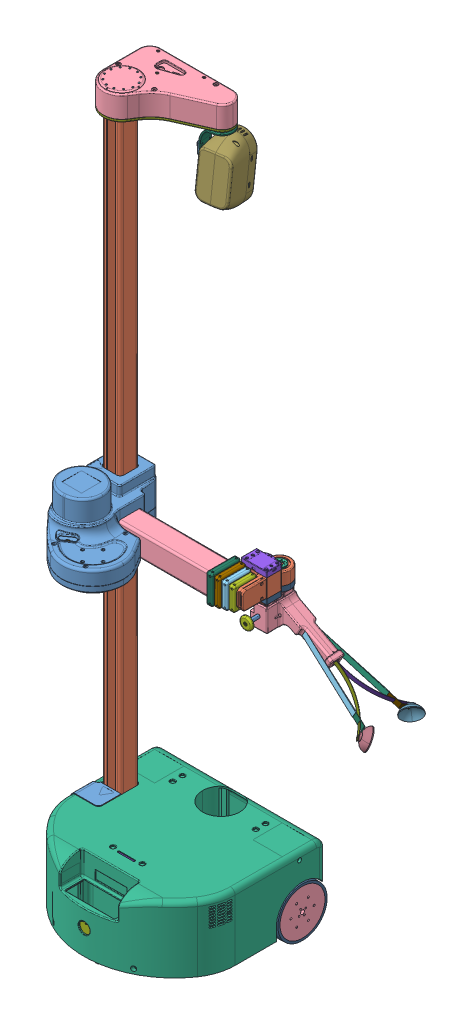
SolidWorks assembly ASM-stretch_re2_nina, configuration Default. Lengths in mm.
Overall size (574.57 1429.23 345.9).
120 component instances, 97 part files, 14 mates.
Components (placement in the parent):
- ASM-base_module.step-1: ASM-base_module.step [Default] at (9.1565 -1330.6492 124.8432) x (1 0 0) z (0 1 0) size (352.17 345.9 1378.51)
  - ASM-base_module1.STEP-1: ASM-base_module1.STEP [Default] at origin size (2.05 13.46 21.35)
  - ASM-base_module2.STEP-1: ASM-base_module2.STEP [Default] at origin size (0.01 36.41 25.92)
  - ASM-base_module3.STEP-1: ASM-base_module3.STEP [Default] at origin size (6.01 6.54 4.61)
  - ASM-base_module4.STEP-1: ASM-base_module4.STEP [Default] at origin size (25.56 91.93 91.93)
  - ASM-base_module5.STEP-1: ASM-base_module5.STEP [Default] at origin size (6 3.9 3.75)
  - ASM-base_module6.STEP-1: ASM-base_module6.STEP [Default] at origin size (352.17 325 150.78)
  - ASM-base_module7.STEP-1: ASM-base_module7.STEP [Default] at origin size (13.8 55.1 43.54)
  - ASM-base_module8.STEP-1: ASM-base_module8.STEP [Default] at origin size (6 3.75 3.9)
  - ASM-base_module9.STEP-1: ASM-base_module9.STEP [Default] at origin size (25.41 123.2 123.2)
  - ASM-base_module10.STEP-1: ASM-base_module10.STEP [Default] at origin size (22.01 60.76 15.75)
  - ASM-base_module11.STEP-1: ASM-base_module11.STEP [Default] at origin size (0.01 35.01 28.06)
  - ASM-base_module12.STEP-1: ASM-base_module12.STEP [Default] at origin size (8.4 7.44 8.82)
  - ASM-base_module13.STEP-1: ASM-base_module13.STEP [Default] at origin size (0.01 35.22 1.01)
  - ASM-base_module14.STEP-1: ASM-base_module14.STEP [Default] at origin size (0.01 20.82 20.37)
  - ASM-base_module15.STEP-1: ASM-base_module15.STEP [Default] at origin size (8.4 6.85 11.7)
  - ASM-base_module16.STEP-1: ASM-base_module16.STEP [Default] at origin size (332.01 319.06 14.35)
  - ASM-base_module17.STEP-1: ASM-base_module17.STEP [Default] at origin size (8.4 7.35 9.57)
  - ASM-base_module18.STEP-1: ASM-base_module18.STEP [Default] at origin size (22.01 60.76 15.75)
  - ASM-base_module19.STEP-1: ASM-base_module19.STEP [Default] at origin size (57.07 47.59 136.87)
  - ASM-base_module20.STEP-1: ASM-base_module20.STEP [Default] at origin size (38.14 38.14 1268.02)
  - ASM-base_module21.STEP-1: ASM-base_module21.STEP [Default] at origin size (25.56 102.18 102.18)
  - ASM-base_module22.STEP-1: ASM-base_module22.STEP [Default] at origin size (27.89 20.39 20.39)
  - ASM-base_module23.STEP-1: ASM-base_module23.STEP [Default] at origin size (8.4 7.6 9.1)
  - ASM-base_module24.STEP-1: ASM-base_module24.STEP [Default] at origin size (6 3.75 3.53)
  - ASM-base_module25.STEP-1: ASM-base_module25.STEP [Default] at origin size (0.01 17.39 23.47)
  - ASM-base_module26.STEP-1: ASM-base_module26.STEP [Default] at origin size (21.07 103.14 103.14)
  - ASM-base_module27.STEP-1: ASM-base_module27.STEP [Default] at origin size (8.4 5.66 7.84)
  - ASM-base_module28.STEP-1: ASM-base_module28.STEP [Default] at origin size (25.41 138.8 138.8)
  - ASM-base_module29.STEP-1: ASM-base_module29.STEP [Default] at origin size (19.01 2.01 2.01)
  - ASM-base_module30.STEP-1: ASM-base_module30.STEP [Default] at origin size (0.01 3.01 115.61)
  - ASM-base_module31.STEP-1: ASM-base_module31.STEP [Default] at origin size (25.49 120.63 120.63)
  - ASM-base_module32.STEP-1: ASM-base_module32.STEP [Default] at origin size (13.8 52.4 43.41)
  - ASM-base_module33.STEP-1: ASM-base_module33.STEP [Default] at origin size (8.4 9.77 9.42)
  - ASM-base_module34.STEP-1: ASM-base_module34.STEP [Default] at origin size (29.85 49.98 45.18)
  - ASM-base_module35.STEP-1: ASM-base_module35.STEP [Default] at origin size (38.71 7.71 0.01)
  - ASM-base_module36.STEP-1: ASM-base_module36.STEP [Default] at origin size (7.64 2.75 7.13)
  - ASM-base_module37.STEP-1: ASM-base_module37.STEP [Default] at origin size (0.01 17.39 23.47)
  - ASM-base_module38.STEP-1: ASM-base_module38.STEP [Default] at origin size (0.01 91.94 91.94)
  - ASM-base_module39.STEP-1: ASM-base_module39.STEP [Default] at origin size (6 3.9 3.75)
- ASM-head_module.STEP-1: ASM-head_module.STEP [Default] at (-30.1698 -72.0673 12.5567) size (192.75 55.42 133.8)
  - SIM-630_head_shell_light_pipes.STEP-1: SIM-630_head_shell_light_pipes.STEP [Default] at (-125.0983 70.6549 49.8978) size (192.75 46.56 133.8)
    - BIG-924_head_shell.STEP-1: BIG-924_head_shell.STEP [Default] at (0 49.7625 0) x (1 0 0) z (0 1 0) size (192.75 133.8 45.8)
    - HDW-923_LightPipe_LFB025CTP.STEP-1: HDW-923_LightPipe_LFB025CTP.STEP [Default] at (-22.9378 51.8 9.4195) x (0 1 0) z (-0.203299 0 0.979117) size (7.11 3.3 3.3)
    - HDW-923_LightPipe_LFB025CTP.STEP-2: HDW-923_LightPipe_LFB025CTP.STEP [Default] at (-6.5158 51.8 -25.8667) x (0 1 0) z (0.471956 0 0.881622) size (7.11 3.3 3.3)
    - HDW-923_LightPipe_LFB025CTP.STEP-3: HDW-923_LightPipe_LFB025CTP.STEP [Default] at (7.7778 51.8 -27.1304) x (0 1 0) z (-0.504358 0 -0.863495) size (7.11 3.3 3.3)
    - HDW-923_LightPipe_LFB025CTP.STEP-4: HDW-923_LightPipe_LFB025CTP.STEP [Default] at (-14.7362 51.8 21.1114) x (0 1 0) z (-0.970654 0 0.24048) size (7.11 3.3 3.3)
    - HDW-923_LightPipe_LFB025CTP.STEP-5: HDW-923_LightPipe_LFB025CTP.STEP [Default] at (-24.1362 51.8 -4.7944) x (0 1 0) z (0.380757 0 0.924675) size (7.11 3.3 3.3)
    - HDW-923_LightPipe_LFB025CTP.STEP-6: HDW-923_LightPipe_LFB025CTP.STEP [Default] at (-18.133 51.8 -17.7146) x (0 1 0) z (0.667843 0 0.744302) size (7.11 3.3 3.3)
    - HDW-923_LightPipe_LFB025CTP.STEP-7: HDW-923_LightPipe_LFB025CTP.STEP [Default] at (28.9074 51.8 -9.4109) x (0 1 0) z (-0.414071 0 0.910245) size (7.11 3.3 3.3)
    - HDW-923_LightPipe_LFB025CTP.STEP-8: HDW-923_LightPipe_LFB025CTP.STEP [Default] at (30.1657 51.8 4.8066) x (0 1 0) z (-0.782358 0 -0.622829) size (7.11 3.3 3.3)
    - HDW-923_LightPipe_LFB025CTP.STEP-9: HDW-923_LightPipe_LFB025CTP.STEP [Default] at (20.693 51.8 -21.1114) x (0 1 0) z (-0.514508 0 -0.857486) size (7.11 3.3 3.3)
    - HDW-923_LightPipe_LFB025CTP.STEP-10: HDW-923_LightPipe_LFB025CTP.STEP [Default] at (24.0898 51.8 17.7146) x (0 1 0) z (-0.414071 0 0.910245) size (7.11 3.3 3.3)
    - HDW-923_LightPipe_LFB025CTP.STEP-11: HDW-923_LightPipe_LFB025CTP.STEP [Default] at (-1.8022 51.8 27.1343) x (0 1 0) z (0.974021 0 0.226458) size (7.11 3.3 3.3)
    - HDW-923_LightPipe_LFB025CTP.STEP-12: HDW-923_LightPipe_LFB025CTP.STEP [Default] at (12.3407 51.8 25.8882) x (0 1 0) z (-0.414071 0 0.910245) size (7.11 3.3 3.3)
    - HDW-A01_5288T111_Oil-Resistant Buna-N Backup Rings_5288T111.STEP-1: HDW-A01_5288T111_Oil-Resistant Buna-N Backup Rings_5288T111.STEP [Default] at (5.1887 44.2723 32.1986) x (-0.310775 0 0.950484) z (0.950484 0 0.310775) size (5.92 1.24 5.92)
    - HDW-A01_5288T111_Oil-Resistant Buna-N Backup Rings_5288T111.STEP-2: HDW-A01_5288T111_Oil-Resistant Buna-N Backup Rings_5288T111.STEP [Default] at (0.8407 44.2723 -32.2627) x (-0.971613 0 0.236575) z (0.236575 0 0.971613) size (5.92 1.24 5.92)
    - HDW-A01_5288T111_Oil-Resistant Buna-N Backup Rings_5288T111.STEP-3: HDW-A01_5288T111_Oil-Resistant Buna-N Backup Rings_5288T111.STEP [Default] at (-29.2159 44.2723 2.142) x (-0.310775 0 0.950484) z (0.950484 0 0.310775) size (5.92 1.24 5.92)
    - HDW-A01_5288T111_Oil-Resistant Buna-N Backup Rings_5288T111.STEP-4: HDW-A01_5288T111_Oil-Resistant Buna-N Backup Rings_5288T111.STEP [Default] at (35.2453 44.2723 -2.2061) x (0.971309 0 0.237823) z (0.237823 0 -0.971309) size (5.92 1.24 5.92)
  - BIG-926_head_bottom_plate_simple.STEP-1: BIG-926_head_bottom_plate_simple.STEP [Default] at (-125.0983 70.6549 49.8978) x (0 0 1) z (0 -1 0) size (133.8 192.72 8.51)
  - HDW-920_head_pan_shaft.STEP-1: HDW-920_head_pan_shaft.STEP [Default] at (9.9017 111.1758 -23.2022) x (0 1 0) z (0.414693 0 0.909961) size (40.5 24.99 24.99)
  - VND-821_head_mount_plate.STEP-1: VND-821_head_mount_plate.STEP [Default] at (-125.0983 70.9908 49.8978) x (0 0 -1) z (0 1 0) size (73.84 73.84 3)
- ASM_head_tilt_hanger.step-1: ASM_head_tilt_hanger.step [Default] at (-5.771 -6.9174 -10.9643) x (0.988973 0 -0.148096) z (0.148096 0 0.988973) size (62.97 69.82 45.01)
  - ASM_head_tilt_hanger1.STEP-1: ASM_head_tilt_hanger1.STEP [Default] at origin size (0.01 1.84 1.84)
  - ASM_head_tilt_hanger2.STEP-1: ASM_head_tilt_hanger2.STEP [Default] at origin size (0.01 1.84 1.84)
  - ASM_head_tilt_hanger3.STEP-1: ASM_head_tilt_hanger3.STEP [Default] at origin size (0.01 1.84 1.84)
  - ASM_head_tilt_hanger4.STEP-1: ASM_head_tilt_hanger4.STEP [Default] at origin size (7.22 2.09 7.22)
  - ASM_head_tilt_hanger5.STEP-1: ASM_head_tilt_hanger5.STEP [Default] at origin size (11.4 31.82 26.47)
  - ASM_head_tilt_hanger6.STEP-1: ASM_head_tilt_hanger6.STEP [Default] at origin size (55.12 69.82 45.01)
  - ASM_head_tilt_hanger7.STEP-1: ASM_head_tilt_hanger7.STEP [Default] at origin size (2.97 6.64 6.64)
  - ASM_head_tilt_hanger8.STEP-1: ASM_head_tilt_hanger8.STEP [Default] at origin size (2.97 6.64 6.64)
  - ASM_head_tilt_hanger9.STEP-1: ASM_head_tilt_hanger9.STEP [Default] at origin size (2.97 6.64 6.64)
- SUB-202_head_tilt_simple.step-1: SUB-202_head_tilt_simple.step [Default] at (-21.5187 -75.739 -52.7585) x (-0.988973 0 0.148096) z (-0.14655 -0.144108 -0.97865) size (65.06 133.38 73.8)
  - SUB-202_head_tilt_simple1.STEP-1: SUB-202_head_tilt_simple1.STEP [Default] at origin size (7.15 7.51 7.51)
  - SUB-202_head_tilt_simple2.STEP-1: SUB-202_head_tilt_simple2.STEP [Default] at origin size (16 81 0.56)
  - SUB-202_head_tilt_simple3.STEP-1: SUB-202_head_tilt_simple3.STEP [Default] at origin size (32.75 27 27)
  - SUB-202_head_tilt_simple4.STEP-1: SUB-202_head_tilt_simple4.STEP [Default] at origin size (3.8 7.01 3.01)
  - SUB-202_head_tilt_simple5.STEP-1: SUB-202_head_tilt_simple5.STEP [Default] at origin size (3.8 7.01 3.01)
  - SUB-202_head_tilt_simple6.STEP-1: SUB-202_head_tilt_simple6.STEP [Default] at origin size (48.91 33.18 33.18)
  - SUB-202_head_tilt_simple7.STEP-1: SUB-202_head_tilt_simple7.STEP [Default] at origin size (3.8 7.01 3.01)
  - SUB-202_head_tilt_simple8.STEP-1: SUB-202_head_tilt_simple8.STEP [Default] at origin size (9.01 6.36 3.19)
  - SUB-202_head_tilt_simple9.STEP-1: SUB-202_head_tilt_simple9.STEP [Default] at origin size (3.8 7.01 3.01)
  - SUB-202_head_tilt_simple10.STEP-1: SUB-202_head_tilt_simple10.STEP [Default] at origin size (56.31 116.27 4.3)
  - SUB-202_head_tilt_simple11.STEP-1: SUB-202_head_tilt_simple11.STEP [Default] at origin size (23.01 2.51 0.01)
  - SUB-202_head_tilt_simple12.STEP-1: SUB-202_head_tilt_simple12.STEP [Default] at origin size (65.06 130.97 69.23)
  - SUB-202_head_tilt_simple13.STEP-1: SUB-202_head_tilt_simple13.STEP [Default] at origin size (39.68 92.75 30.1)
  - SUB-202_head_tilt_simple14.STEP-1: SUB-202_head_tilt_simple14.STEP [Default] at origin size (27.52 27.52 27.52)
- ASM_Arm_with_Wrist_simple.step-1: ASM_Arm_with_Wrist_simple.step [Default] at (-123.1677 -699.0905 99.7103) size (377.58 155.09 260.45)
  - ASM_Arm_with_Wrist_simple1.STEP-1: ASM_Arm_with_Wrist_simple1.STEP [Default] at origin size (13.01 59.49 59.46)
  - ASM_Arm_with_Wrist_simple2.STEP-1: ASM_Arm_with_Wrist_simple2.STEP [Default] at origin size (100.01 4.01 96.01)
  - ASM_Arm_with_Wrist_simple3.STEP-1: ASM_Arm_with_Wrist_simple3.STEP [Default] at origin size (0.01 34.01 34.01)
  - ASM_Arm_with_Wrist_simple4.STEP-1: ASM_Arm_with_Wrist_simple4.STEP [Default] at origin size (10.01 0.01 10.01)
  - ASM_Arm_with_Wrist_simple5.STEP-1: ASM_Arm_with_Wrist_simple5.STEP [Default] at origin size (191.75 155.09 244.07)
  - ASM_Arm_with_Wrist_simple6.STEP-1: ASM_Arm_with_Wrist_simple6.STEP [Default] at origin size (78.93 57.83 130.52)
  - ASM_Arm_with_Wrist_simple7.STEP-1: ASM_Arm_with_Wrist_simple7.STEP [Default] at origin size (177.19 121.67 235.79)
  - ASM_Arm_with_Wrist_simple8.STEP-1: ASM_Arm_with_Wrist_simple8.STEP [Default] at origin size (244.12 74.4 74.4)
  - ASM_Arm_with_Wrist_simple9.STEP-1: ASM_Arm_with_Wrist_simple9.STEP [Default] at origin size (13.01 51.36 51.36)
  - ASM_Arm_with_Wrist_simple10.STEP-1: ASM_Arm_with_Wrist_simple10.STEP [Default] at origin size (32.66 43.09 32.66)
  - ASM_Arm_with_Wrist_simple11.STEP-1: ASM_Arm_with_Wrist_simple11.STEP [Default] at origin size (13.01 47.36 47.36)
  - ASM_Arm_with_Wrist_simple12.STEP-1: ASM_Arm_with_Wrist_simple12.STEP [Default] at origin size (52.51 20.59 50.95)
  - ASM_Arm_with_Wrist_simple13.STEP-1: ASM_Arm_with_Wrist_simple13.STEP [Default] at origin size (13.01 55.26 55.26)
  - ASM_Arm_with_Wrist_simple14.STEP-1: ASM_Arm_with_Wrist_simple14.STEP [Default] at origin size (53.78 12.96 73.76)
- HDW-911_gripper_mount_bracket.STEP-1: HDW-911_gripper_mount_bracket.STEP [Default] at (123.1348 -627.1623 -27.3033) x (0 1 0) z (0.027951 0 0.999609) size (14 28 56.75)
  - VND-817_gripper_mount_bracket.STEP-1: VND-817_gripper_mount_bracket.STEP [Default] at (-122.2701 -0.2167 85.7868) size (11.5 28 56.75)
  - VND-818_MPP-1.5mm-4-PennEngineering.STEP-1: VND-818_MPP-1.5mm-4-PennEngineering.STEP [Default] at (-104.2701 -7.335 37.0133) size (4 2.24 2.24)
  - VND-818_MPP-1.5mm-4-PennEngineering.STEP-2: VND-818_MPP-1.5mm-4-PennEngineering.STEP [Default] at (-104.2701 -7.335 51.0603) size (4 2.24 2.24)
- ASM-207_Gripper_Simple.step-1: ASM-207_Gripper_Simple.step [Default] at (251.416 -808.1884 -3.9687) x (0.999609 0 -0.027951) z (0.027951 0 0.999609) size (261.51 171.11 139.86)
  - ASM-207_Gripper_Simple1.STEP-1: ASM-207_Gripper_Simple1.STEP [Default] at origin size (35.66 45.77 42.41)
  - ASM-207_Gripper_Simple2.STEP-1: ASM-207_Gripper_Simple2.STEP [Default] at origin size (38.03 42.61 42.49)
  - ASM-207_Gripper_Simple3.STEP-1: ASM-207_Gripper_Simple3.STEP [Default] at origin size (167.87 105.91 44.86)
  - ASM-207_Gripper_Simple4.STEP-1: ASM-207_Gripper_Simple4.STEP [Default] at origin size (111.68 70.98 65.43)
  - ASM-207_Gripper_Simple5.STEP-1: ASM-207_Gripper_Simple5.STEP [Default] at origin size (111.76 70.98 65.24)
  - ASM-207_Gripper_Simple6.STEP-1: ASM-207_Gripper_Simple6.STEP [Default] at origin size (168.93 105.91 49.34)
  - ASM-207_Gripper_Simple7.STEP-1: ASM-207_Gripper_Simple7.STEP [Default] at origin size (7.49 7.49 25.15)
  - ASM-207_Gripper_Simple8.STEP-1: ASM-207_Gripper_Simple8.STEP [Default] at origin size (0.65 0.01 4.01)
  - ASM-207_Gripper_Simple9.STEP-1: ASM-207_Gripper_Simple9.STEP [Default] at origin size (0.65 0.65 0.01)
  - ASM-207_Gripper_Simple10.STEP-1: ASM-207_Gripper_Simple10.STEP [Default] at origin size (141.61 96.71 65.91)
  - ASM-207_Gripper_Simple11.STEP-1: ASM-207_Gripper_Simple11.STEP [Default] at origin size (144.09 94.9 39.31)
  - ASM-207_Gripper_Simple12.STEP-1: ASM-207_Gripper_Simple12.STEP [Default] at origin size (144.09 94.9 38.54)
  - ASM-207_Gripper_Simple13.STEP-1: ASM-207_Gripper_Simple13.STEP [Default] at origin size (25.66 25.66 5.66)
Mates (geometry in assembly coordinates):
- Concentric4: concentric: cylinder of ASM-base_module.step-1/ASM-base_module20.STEP-1 through (-169.2181 -1266.0765 47.2919) axis (0 1 0) radius 2.1; cylinder of ASM-head_module.STEP-1/VND-821_head_mount_plate.STEP-1 through (-169.2181 -1.0765 47.2919) axis (0 1 0) radius 2.6
- Concentric5: concentric: cylinder of ASM-base_module.step-1/ASM-base_module20.STEP-1 through (-141.3181 -1266.0765 77.6173) axis (0 1 0) radius 2.1; cylinder of ASM-head_module.STEP-1/VND-821_head_mount_plate.STEP-1 through (-141.3181 -1.0765 77.6173) axis (0 1 0) radius 2.6
- Coincident2: coincident: plane of ASM-base_module.step-1/ASM-base_module20.STEP-1 through (-160.5181 -1.0765 55.3919) normal (0 1 0); plane of ASM-head_module.STEP-1/VND-821_head_mount_plate.STEP-1 through (-142.1744 -1.0765 75.5483) normal (0 -1 0)
- Concentric6: concentric: cylinder of ASM-head_module.STEP-1/HDW-920_head_pan_shaft.STEP-1 through (-20.2681 -6.2727 -10.6454) axis (0 1 0) radius 12.495; cylinder of ASM_head_tilt_hanger.step-1/ASM_head_tilt_hanger6.STEP-1 through (-20.2681 -2.2727 -10.6454) axis (0 -1 0) radius 13.495
- Coincident3: coincident: plane of ASM-head_module.STEP-1/HDW-920_head_pan_shaft.STEP-1 through (-20.2681 -4.2727 -10.6454) normal (0 -1 0); plane of ASM_head_tilt_hanger.step-1/ASM_head_tilt_hanger6.STEP-1 through (-20.2681 -4.2727 -10.6454) normal (0 1 0)
- Concentric7: concentric: cylinder of ASM_head_tilt_hanger.step-1/ASM_head_tilt_hanger6.STEP-1 through (-50.4989 -57.5835 -4.804) axis (0.988973 0 -0.148096) radius 12.5; cylinder of SUB-202_head_tilt_simple.step-1/SUB-202_head_tilt_simple6.STEP-1 through (-47.532 -57.5835 -5.2482) axis (0.988973 0 -0.148096) radius 12.5
- Coincident4: coincident: plane of ASM_head_tilt_hanger.step-1/ASM_head_tilt_hanger6.STEP-1 through (-47.532 -57.5835 -5.2482) normal (0.988973 0 -0.148096); plane of SUB-202_head_tilt_simple.step-1/SUB-202_head_tilt_simple6.STEP-1 through (-47.532 -57.5835 -5.2482) normal (-0.988973 0 0.148096)
- Distance1: distance = 1.5 mm: plane of ASM-base_module.step-1/ASM-base_module20.STEP-1 through (-136.2054 -1266.0765 75.5483) normal (1 0 0); plane of ASM_Arm_with_Wrist_simple.step-1/ASM_Arm_with_Wrist_simple5.STEP-1 through (-134.7054 -640.7416 49.4609) normal (-1 0 0)
- Distance2: distance = 1.5 mm: plane of ASM-base_module.step-1/ASM-base_module20.STEP-1 through (-142.1744 -1266.0765 43.3919) normal (0 0 -1); plane of ASM_Arm_with_Wrist_simple.step-1/ASM_Arm_with_Wrist_simple5.STEP-1 through (-168.4664 -640.7416 41.8919) normal (0 0 1)
- Concentric8: concentric: cylinder of ASM_Arm_with_Wrist_simple.step-1/ASM_Arm_with_Wrist_simple10.STEP-1 through (124.5823 -729.9325 16.7103) axis (0 1 0) radius 5.5; cylinder of HDW-911_gripper_mount_bracket.STEP-1/VND-817_gripper_mount_bracket.STEP-1 through (124.5823 -731.4325 16.7103) axis (0 1 0) radius 5.5
- Coincident5: coincident: plane of ASM_Arm_with_Wrist_simple.step-1/ASM_Arm_with_Wrist_simple10.STEP-1 through (124.5823 -729.9325 16.7103) normal (0 -1 0); plane of HDW-911_gripper_mount_bracket.STEP-1/VND-817_gripper_mount_bracket.STEP-1 through (125.7492 -729.9325 58.444) normal (0 1 0)
- Concentric9: concentric: cylinder of HDW-911_gripper_mount_bracket.STEP-1/VND-817_gripper_mount_bracket.STEP-1 through (135.1587 -738.4325 1.4087) axis (-0.027951 0 -0.999609) radius 1.45; cylinder of ASM-207_Gripper_Simple.step-1/ASM-207_Gripper_Simple10.STEP-1 through (134.8673 -738.4325 -9.0142) axis (-0.027951 0 -0.999609) radius 1.35
- Concentric10: concentric: cylinder of HDW-911_gripper_mount_bracket.STEP-1/VND-817_gripper_mount_bracket.STEP-1 through (113.1673 -738.4325 2.0236) axis (-0.027951 0 -0.999609) radius 1.45; cylinder of ASM-207_Gripper_Simple.step-1/ASM-207_Gripper_Simple10.STEP-1 through (112.8759 -738.4325 -8.3993) axis (-0.027951 0 -0.999609) radius 1.35
- Coincident6: coincident: plane of HDW-911_gripper_mount_bracket.STEP-1/VND-817_gripper_mount_bracket.STEP-1 through (124.2049 -749.4325 3.2156) normal (0.027951 0 0.999609); plane of ASM-207_Gripper_Simple.step-1/ASM-207_Gripper_Simple10.STEP-1 through (136.7001 -703.6299 2.8662) normal (0.027951 0 0.999609)
